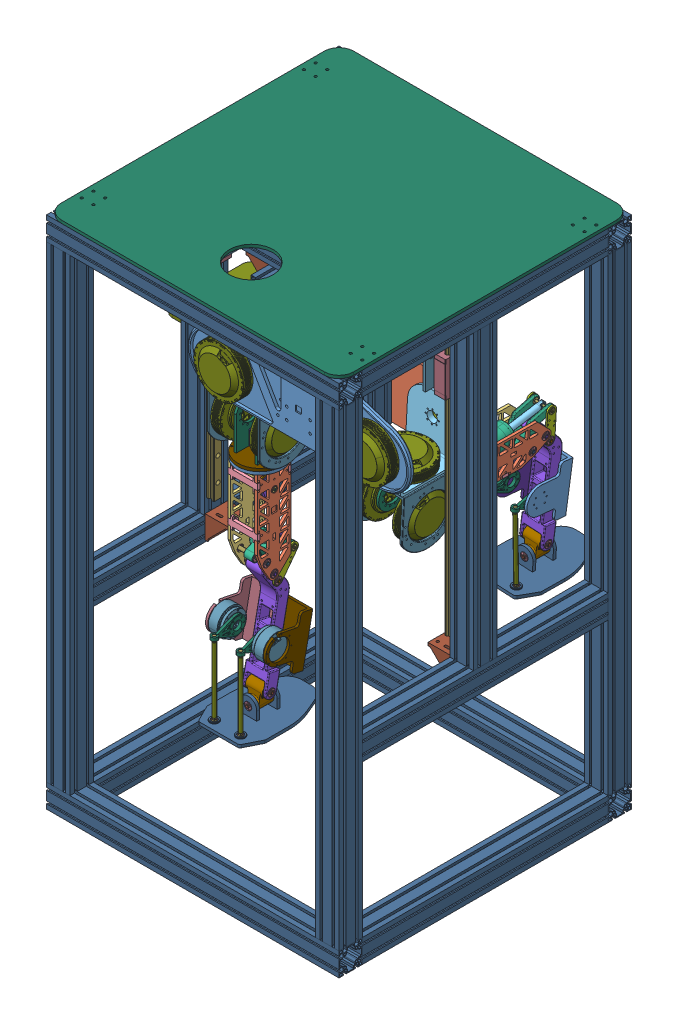
SolidWorks assembly 完整下肢, configuration 默认. Lengths in mm. (continued)
Mates (geometry in assembly coordinates): (continued)
- 重合58: coincident anti-aligned: plane of 腿髋转接架侧板V2-4 through (-333.8233 -333.6825 700.2525) normal (0 -1 0); plane of 腿髋转接架底座V2-2 through (-301.8233 -333.6825 652.2525) normal (0 1 0)
- 同心49: concentric aligned: cylinder of 腿髋转接架侧板V2-1 through (225.0525 -200.9494 601.8455) axis (-0.000625 -0.011709 -0.999931) radius 2.75; cylinder of 腿髋转接架底座V2-1 through (225.0318 -201.3358 568.8478) axis (-0.000625 -0.011709 -0.999931) radius 2.75
- 同心50: concentric aligned: cylinder of 腿髋转接架侧板V2-2 through (149.4212 -267.0042 602.6663) axis (-0.000625 -0.011709 -0.999931) radius 2.75; cylinder of 腿髋转接架底座V2-1 through (149.4006 -267.3906 569.6686) axis (-0.000625 -0.011709 -0.999931) radius 2.75
- 同心51: concentric aligned: cylinder of 腿髋转接架侧板V2-3 through (-265.8233 -283.6825 617.2525) axis (0 -1 0) radius 2.75; cylinder of 腿髋转接架底座V2-2 through (-265.8233 -316.6825 617.2525) axis (0 -1 0) radius 2.75
- 同心53: concentric aligned: cylinder of 腿髋转接架侧板V2-4 through (-337.8233 -283.6825 687.2525) axis (0 -1 0) radius 2.75; cylinder of 腿髋转接架底座V2-2 through (-337.8233 -316.6825 687.2525) axis (0 -1 0) radius 2.75
- 重合59: coincident anti-aligned: plane of 腿髋转接架侧板V2-3 through (-269.8233 -333.6825 604.2525) normal (0 -1 0); plane of 腿髋转接架底座V2-2 through (-301.8233 -333.6825 652.2525) normal (0 1 0)
- 重合61: coincident anti-aligned: plane of 腿髋转接架底座V2-2 through (-301.8233 -343.6825 652.2525) normal (0 -1 0); plane of 大腿主干_上板V2-1 through (-301.8233 -343.6825 652.2525) normal (0 1 0)
- 同心54: concentric anti-aligned: cylinder of 腿髋转接架底座V2-2 through (-301.8233 -343.6825 652.2525) axis (0 1 0) radius 75; cylinder of 大腿主干_上板V2-1 through (-301.8233 -343.6825 652.2525) axis (0 -1 0) radius 75
- 同心55: concentric aligned: cylinder of 腿髋转接架底座V2-2 through (-322.8233 -316.6825 652.2525) axis (0 -1 0) radius 2.75; cylinder of 大腿主干_上板V2-1 through (-322.8233 -343.6825 652.2525) axis (0 -1 0) radius 2.5
- 重合62: coincident anti-aligned: plane of 腿髋转接架底座V2-1 through (187.1993 -234.6794 542.26) normal (-0.000625 -0.011709 -0.999931); plane of 大腿主干_上板V2-2 through (187.1993 -234.6794 542.26) normal (0.000625 0.011709 0.999931)
- 同心56: concentric anti-aligned: cylinder of 腿髋转接架底座V2-1 through (187.1993 -234.6794 542.26) axis (0.000625 0.011709 0.999931) radius 75; cylinder of 大腿主干_上板V2-2 through (187.1993 -234.6794 542.26) axis (-0.000625 -0.011709 -0.999931) radius 75
- 同心57: concentric aligned: cylinder of 腿髋转接架底座V2-1 through (208.1863 -235.4834 569.2582) axis (-0.000625 -0.011709 -0.999931) radius 2.75; cylinder of 大腿主干_上板V2-2 through (208.1694 -235.7996 542.26) axis (-0.000625 -0.011709 -0.999931) radius 2.75
- 重合63: coincident anti-aligned: plane of 大腿主干_上板V2-2 through (187.1931 -234.7964 532.2607) normal (-0.000625 -0.011709 -0.999931); plane of 大腿主干_右侧板V2-1 through (-197.0913 -196.244 532.0497) normal (0.000625 0.011709 0.999931)
- 同心58: concentric anti-aligned: cylinder of 大腿主干_上板V2-2 through (233.968 -212.1438 541.9669) axis (-0.000625 -0.011709 -0.999931) radius 2.75; cylinder of 大腿主干_右侧板V2-1 through (233.948 -212.5184 509.9691) axis (0.000625 0.011709 0.999931) radius 2.5
- 同心59: concentric anti-aligned: cylinder of 大腿主干_上板V2-2 through (231.3011 -262.0691 542.5532) axis (-0.000625 -0.011709 -0.999931) radius 2.75; cylinder of 大腿主干_右侧板V2-1 through (231.281 -262.4438 510.5554) axis (0.000625 0.011709 0.999931) radius 2.5
- 重合64: coincident anti-aligned: plane of 大腿主干_上板V2-1 through (-301.8233 -353.6825 652.2525) normal (0 -1 0); plane of 大腿主干_右侧板V2-2 through (-687.617 -353.6825 634.2525) normal (0 1 0)
- 同心61: concentric anti-aligned: cylinder of 大腿主干_上板V2-1 through (-256.3233 -343.6825 627.2525) axis (0 -1 0) radius 2.75; cylinder of 大腿主干_右侧板V2-2 through (-256.3233 -375.6825 627.2525) axis (0 1 0) radius 2.5
- 同心62: concentric anti-aligned: line of 大腿主干_上板V2-1 through (-256.3233 -343.6825 677.2525) axis (0 -1 0); axis of 大腿主干_右侧板V2-2 through (-256.3233 -363.6825 677.2525) axis (0 1 0)
- 重合65: coincident anti-aligned: plane of 大腿主干_上板V2-2 through (187.1931 -234.7964 532.2607) normal (-0.000625 -0.011709 -0.999931); plane of 大腿主干_左侧板V2-1 through (-201.1451 -272.1306 532.9408) normal (0.000625 0.011709 0.999931)
- 同心63: concentric anti-aligned: cylinder of 大腿主干_上板V2-2 through (143.0976 -207.2896 541.9669) axis (-0.000625 -0.011709 -0.999931) radius 2.75; cylinder of 大腿主干_左侧板V2-1 through (143.0807 -207.6057 514.9688) axis (0.000625 0.011709 0.999931) radius 2.5
- 同心64: concentric anti-aligned: cylinder of 大腿主干_上板V2-2 through (140.4306 -257.2149 542.5532) axis (-0.000625 -0.011709 -0.999931) radius 2.75; cylinder of 大腿主干_左侧板V2-1 through (140.4137 -257.5311 515.555) axis (0.000625 0.011709 0.999931) radius 2.5
- 重合66: coincident anti-aligned: plane of 大腿主干_上板V2-1 through (-301.8233 -353.6825 652.2525) normal (0 -1 0); plane of 大腿主干_左侧板V2-2 through (-687.617 -353.6825 710.2525) normal (0 1 0)
- 同心65: concentric anti-aligned: cylinder of 大腿主干_上板V2-1 through (-347.3233 -343.6825 627.2525) axis (0 -1 0) radius 2.75; cylinder of 大腿主干_左侧板V2-2 through (-347.3233 -370.6825 627.2525) axis (0 1 0) radius 2.5
- 同心66: concentric anti-aligned: cylinder of 大腿主干_上板V2-1 through (-347.3233 -343.6825 677.2525) axis (0 -1 0) radius 2.75; circle of 大腿主干_左侧板V2-2
- 重合67: coincident anti-aligned: plane of 大腿主干_左侧板V2-1 through (109.5394 -282.471 212.8456) normal (-0.053339 -0.998508 0.011726); plane of 大腿侧板连接V2-4 through (134.6758 -280.5846 487.8267) normal (0.053339 0.998508 -0.011726)
- 重合68: coincident anti-aligned: plane of 大腿主干_左侧板V2-1 through (112.2717 -231.3226 487.2638) normal (0.000625 0.011709 0.999931); plane of 大腿侧板连接V2-4 through (134.1424 -290.5696 487.9439) normal (-0.000625 -0.011709 -0.999931)
- 重合69: coincident anti-aligned: plane of 大腿主干_左侧板V2-1 through (143.1703 -290.2887 552.9394) normal (0.998576 -0.053343 0); plane of 大腿侧板连接V2-4 through (143.1296 -291.0497 487.9439) normal (-0.998576 0.053343 0)
- 重合70: coincident anti-aligned: plane of 大腿主干_左侧板V2-1 through (109.5394 -282.471 212.8456) normal (-0.053339 -0.998508 0.011726); plane of 大腿侧板连接V2-1 through (134.5818 -282.3444 337.5398) normal (0.053339 0.998508 -0.011726)
- 重合71: coincident anti-aligned: plane of 大腿主干_左侧板V2-1 through (112.1777 -233.0825 336.977) normal (0.000625 0.011709 0.999931); plane of 大腿侧板连接V2-1 through (134.0484 -292.3295 337.6571) normal (-0.000625 -0.011709 -0.999931)
- 重合72: coincident anti-aligned: plane of 大腿主干_左侧板V2-1 through (143.1703 -290.2887 552.9394) normal (0.998576 -0.053343 0); plane of 大腿侧板连接V2-1 through (143.0356 -292.8096 337.6571) normal (-0.998576 0.053343 0)
- 重合74: coincident anti-aligned: plane of 大腿主干_左侧板V2-1 through (114.8445 -183.1601 506.6996) normal (0.053339 0.998508 -0.011726); plane of 大腿侧板连接V2-5 through (139.8089 -184.4937 506.6996) normal (-0.053339 -0.998508 0.011726)
- 重合75: coincident anti-aligned: plane of 大腿主干_左侧板V2-1 through (115.3654 -173.4092 486.5837) normal (0.000625 0.011709 0.999931); plane of 大腿侧板连接V2-5 through (140.3298 -174.7428 486.5837) normal (-0.000625 -0.011709 -0.999931)
- 重合76: coincident anti-aligned: plane of 大腿主干_左侧板V2-1 through (143.1703 -290.2887 552.9394) normal (0.998576 -0.053343 0); plane of 大腿侧板连接V2-5 through (149.3295 -174.9887 506.5824) normal (-0.998576 0.053343 0)
- 重合77: coincident anti-aligned: plane of 大腿主干_左侧板V2-2 through (-376.8233 -378.6825 604.2525) normal (0 0 -1); plane of 大腿侧板连接V2-2 through (-251.8233 -398.6825 604.2525) normal (0 0 1)
- 重合78: coincident anti-aligned: plane of 大腿主干_左侧板V2-2 through (-376.8233 -398.6825 594.2525) normal (0 1 0); plane of 大腿侧板连接V2-2 through (-251.8233 -398.6825 594.2525) normal (0 -1 0)
- 重合79: coincident anti-aligned: plane of 大腿主干_左侧板V2-2 through (-342.8233 -333.6825 710.2525) normal (1 0 0); plane of 大腿侧板连接V2-2 through (-342.8233 -398.6825 594.2525) normal (-1 0 0)
- 重合80: coincident anti-aligned: plane of 大腿主干_左侧板V2-2 through (-376.8233 -673.6825 700.2525) normal (0 0 1); plane of 大腿侧板连接V2-6 through (-351.8233 -398.6825 700.2525) normal (0 0 -1)
- 重合81: coincident anti-aligned: plane of 大腿主干_左侧板V2-2 through (-376.8233 -398.6825 652.2525) normal (0 1 0); plane of 大腿侧板连接V2-6 through (-351.8233 -398.6825 710.2525) normal (0 -1 0)
- 重合82: coincident anti-aligned: plane of 大腿主干_左侧板V2-2 through (-342.8233 -333.6825 710.2525) normal (1 0 0); plane of 大腿侧板连接V2-6 through (-342.8233 -398.6825 710.2525) normal (-1 0 0)
- 重合83: coincident anti-aligned: plane of 大腿主干_左侧板V2-2 through (-376.8233 -673.6825 700.2525) normal (0 0 1); plane of 大腿侧板连接V2-3 through (-351.8233 -548.9797 700.2525) normal (0 0 -1)
- 重合84: coincident anti-aligned: plane of 大腿主干_左侧板V2-2 through (-376.8233 -548.9797 652.2525) normal (0 1 0); plane of 大腿侧板连接V2-3 through (-351.8233 -548.9797 710.2525) normal (0 -1 0)
- 重合85: coincident anti-aligned: plane of 大腿主干_左侧板V2-2 through (-342.8233 -333.6825 710.2525) normal (1 0 0); plane of 大腿侧板连接V2-3 through (-342.8233 -548.9797 710.2525) normal (-1 0 0)
- 重合86: coincident anti-aligned: plane of 大腿主干_上板V2-1 through (-301.8233 -353.6825 652.2525) normal (0 -1 0); plane of 大腿主干_连接块-3 through (-302.8233 -353.6825 647.2525) normal (0 1 0)
- 重合87: coincident anti-aligned: plane of 大腿主干_左侧板V2-2 through (-342.8233 -333.6825 710.2525) normal (1 0 0); plane of 大腿主干_连接块-3 through (-342.8233 -353.6825 647.2525) normal (-1 0 0)
- 重合88: coincident anti-aligned: plane of 大腿主干_上板V2-1 through (-301.8233 -353.6825 652.2525) normal (0 -1 0); plane of 大腿主干_连接块-4 through (-300.8233 -353.6825 657.2525) normal (0 1 0)
- 重合89: coincident anti-aligned: plane of 大腿主干_右侧板V2-2 through (-260.8233 -333.6825 710.2525) normal (-1 0 0); plane of 大腿主干_连接块-4 through (-260.8233 -353.6825 657.2525) normal (1 0 0)
- 重合90: coincident anti-aligned: plane of 大腿主干_上板V2-2 through (187.1931 -234.7964 532.2607) normal (-0.000625 -0.011709 -0.999931); plane of 大腿主干_连接块-1 through (187.9249 -239.8423 532.3194) normal (0.000625 0.011709 0.999931)
- 重合91: coincident anti-aligned: plane of 大腿主干_右侧板V2-1 through (225.0535 -294.6628 552.9394) normal (-0.998576 0.053343 0); plane of 大腿主干_连接块-1 through (227.868 -241.976 532.3194) normal (0.998576 -0.053343 0)
- 重合93: coincident anti-aligned: plane of 大腿主干_上板V2-2 through (187.1931 -234.7964 532.2607) normal (-0.000625 -0.011709 -0.999931); plane of 大腿主干_连接块-2 through (186.4612 -229.7506 532.2021) normal (0.000625 0.011709 0.999931)
- 重合94: coincident anti-aligned: plane of 大腿主干_左侧板V2-1 through (143.1703 -290.2887 552.9394) normal (0.998576 -0.053343 0); plane of 大腿主干_连接块-2 through (146.5181 -227.6169 532.2021) normal (-0.998576 0.053343 0)
- 同心67: concentric anti-aligned: cylinder of 大腿主干_连接块-2 through (166.2004 -234.0978 496.2632) axis (0.000625 0.011709 0.999931) radius 2.5; cylinder of 大腿主干_上板V2-2 through (166.2292 -233.5592 542.26) axis (-0.000625 -0.011709 -0.999931) radius 2.5
- 同心68: concentric anti-aligned: cylinder of 大腿主干_上板V2-2 through (208.1694 -235.7996 542.26) axis (-0.000625 -0.011709 -0.999931) radius 2.75; cylinder of 大腿主干_连接块-1 through (208.1406 -236.3382 496.2632) axis (0.000625 0.011709 0.999931) radius 2.5
- 同心69: concentric anti-aligned: cylinder of 大腿主干_上板V2-1 through (-280.8233 -343.6825 652.2525) axis (0 -1 0) radius 2.75; cylinder of 大腿主干_连接块-4 through (-280.8233 -389.6825 652.2525) axis (0 1 0) radius 2.5
- 同心70: concentric anti-aligned: cylinder of 大腿主干_上板V2-1 through (-322.8233 -343.6825 652.2525) axis (0 -1 0) radius 2.5; cylinder of 大腿主干_连接块-3 through (-322.8233 -389.6825 652.2525) axis (0 1 0) radius 2.5
- 同心71: concentric aligned: cylinder of 大腿主干_左侧板V2-2 through (-238.8233 -423.6825 652.2525) axis (-1 0 0) radius 9.5; cylinder of 轴承_NSK635-4 through (-351.4346 -423.6825 652.2525) axis (-1 0 0) radius 9.5
- 重合95: coincident anti-aligned: plane of 大腿主干_左侧板V2-2 through (-352.8233 -432.1825 652.2525) normal (1 0 0); plane of 轴承_NSK635-4 through (-352.8233 -414.2003 651.6711) normal (-1 0 0)
- 同心72: concentric aligned: cylinder of 大腿主干_右侧板V2-2 through (-238.8233 -423.6825 652.2525) axis (-1 0 0) radius 9.5; cylinder of 轴承_NSK635-2 through (-255.4346 -423.6825 652.2525) axis (-1 0 0) radius 9.5
- 重合96: coincident anti-aligned: plane of 大腿主干_右侧板V2-2 through (-250.8233 -432.1825 652.2525) normal (-1 0 0); plane of 轴承_NSK635-2 through (-250.8233 -415.6975 651.7629) normal (1 0 0)
- 同心73: concentric aligned: cylinder of 大腿主干_右侧板V2-1 through (250.0596 -238.9767 462.2655) axis (-0.998576 0.053343 0) radius 9.5; cylinder of 轴承_NSK635-1 through (233.4719 -238.0906 462.2655) axis (-0.998576 0.053343 0) radius 9.5
- 重合97: coincident anti-aligned: plane of 大腿主干_右侧板V2-1 through (238.0714 -238.4361 453.7661) normal (-0.998576 0.053343 0); plane of 轴承_NSK635-1 through (238.4707 -230.9596 465.3357) normal (0.998576 -0.053343 0)
- 同心74: concentric aligned: cylinder of 大腿主干_左侧板V2-1 through (250.0596 -238.9767 462.2655) axis (-0.998576 0.053343 0) radius 9.5; cylinder of 轴承_NSK635-3 through (137.6086 -232.9697 462.2655) axis (-0.998576 0.053343 0) radius 9.5
- 重合98: coincident anti-aligned: plane of 大腿主干_左侧板V2-1 through (136.2166 -232.9951 453.7661) normal (0.998576 -0.053343 0); plane of 轴承_NSK635-3 through (136.6898 -224.1355 465.9114) normal (-0.998576 0.053343 0)
- 同心75: concentric anti-aligned: cylinder of 轴承_NSK635-1 through (233.4719 -238.0906 462.2655) axis (-0.998576 0.053343 0) radius 2.5; cylinder of 大腿_电机轴-1 through (133.2262 -232.7356 462.2655) axis (0.998576 -0.053343 0) radius 2.5
- 距离3: distance = 3 mm aligned: plane of 大腿_电机轴-1 through (241.0724 -238.4966 462.2655) normal (0.998576 -0.053343 0); plane of 轴承_NSK635-1 through (238.1998 -236.0313 463.225) normal (0.998576 -0.053343 0)
- 同心76: concentric anti-aligned: cylinder of 轴承_NSK635-4 through (-351.4346 -423.6825 652.2525) axis (-1 0 0) radius 2.5; cylinder of 大腿_电机轴-2 through (-355.8233 -423.6825 652.2525) axis (1 0 0) radius 2.5
- 距离4: distance = 3 mm aligned: plane of 轴承_NSK635-4 through (-352.8233 -419.69 652.0077) normal (-1 0 0); plane of 大腿_电机轴-2 through (-355.8233 -423.6825 652.2525) normal (-1 0 0)
- 同心77: concentric anti-aligned: cylinder of 大腿_电机轴-2 through (-355.8233 -423.6825 652.2525) axis (1 0 0) radius 2.5; cylinder of 轴套-5 through (-256.8233 -423.6825 652.2525) axis (-1 0 0) radius 2.5
- 重合101: coincident anti-aligned: plane of 轴承_NSK635-2 through (-256.8233 -419.69 652.0077) normal (-1 0 0); plane of 轴套-5 through (-256.8233 -423.6825 652.2525) normal (1 0 0)
- 同心78: concentric anti-aligned: cylinder of 大腿_电机轴-2 through (-355.8233 -423.6825 652.2525) axis (1 0 0) radius 2.5; cylinder of 轴套-6 through (-306.3233 -423.6825 652.2525) axis (-1 0 0) radius 2.5
- 重合102: coincident anti-aligned: plane of 轴承_NSK635-4 through (-346.8233 -421.1872 652.0995) normal (1 0 0); plane of 轴套-6 through (-346.8233 -423.6825 652.2525) normal (-1 0 0)
- 同心79: concentric aligned: cylinder of 大腿_电机轴-1 through (133.2262 -232.7356 462.2655) axis (0.998576 -0.053343 0) radius 2.5; cylinder of 轴套-4 through (191.6429 -235.8561 462.2655) axis (0.998576 -0.053343 0) radius 2.5
- 重合103: coincident anti-aligned: plane of 轴承_NSK635-1 through (232.2822 -234.328 463.8006) normal (-0.998576 0.053343 0); plane of 轴套-4 through (232.0852 -238.0165 462.2655) normal (0.998576 -0.053343 0)
- 同心80: concentric aligned: cylinder of 大腿_电机轴-1 through (133.2262 -232.7356 462.2655) axis (0.998576 -0.053343 0) radius 2.5; cylinder of 轴套-3 through (142.2133 -233.2156 462.2655) axis (0.998576 -0.053343 0) radius 2.5
- 重合104: coincident anti-aligned: plane of 轴承_NSK635-3 through (142.3365 -230.9104 463.225) normal (0.998576 -0.053343 0); plane of 轴套-3 through (142.2133 -233.2156 462.2655) normal (-0.998576 0.053343 0)
- 同心81: concentric anti-aligned: cylinder of 大腿主干_右侧板V2-1 through (335.5213 -271.003 255.8742) axis (-0.998576 0.053343 0) radius 11; cylinder of 轴承_NSK6900NR-5 through (235.2272 -265.6454 255.8742) axis (0.998576 -0.053343 0) radius 11
- 重合105: coincident anti-aligned: plane of 大腿主干_右侧板V2-1 through (234.8664 -265.6261 255.8742) normal (0.998576 -0.053343 0); plane of 轴承_NSK6900NR-5 through (234.8664 -265.6261 255.8742) normal (-0.998576 0.053343 0)
- 同心82: concentric aligned: cylinder of 大腿主干_右侧板V2-1 through (137.0641 -235.8762 212.2827) axis (0.998576 -0.053343 0) radius 11; cylinder of 轴承_NSK6900NR-6 through (236.5336 -241.1897 212.2827) axis (0.998576 -0.053343 0) radius 11
- 重合106: coincident anti-aligned: plane of 大腿主干_右侧板V2-1 through (236.1728 -241.1704 212.2827) normal (0.998576 -0.053343 0); plane of 轴承_NSK6900NR-6 through (236.1728 -241.1704 212.2827) normal (-0.998576 0.053343 0)
- 同心83: concentric aligned: cylinder of 大腿主干_左侧板V2-1 through (335.5213 -271.003 255.8742) axis (-0.998576 0.053343 0) radius 11; cylinder of 轴承_NSK6900NR-8 through (136.1459 -260.3526 255.8742) axis (-0.998576 0.053343 0) radius 11
- 重合107: coincident anti-aligned: plane of 大腿主干_左侧板V2-1 through (136.5066 -260.3719 255.8742) normal (-0.998576 0.053343 0); plane of 轴承_NSK6900NR-8 through (136.5066 -260.3719 255.8742) normal (0.998576 -0.053343 0)
- 同心84: concentric anti-aligned: cylinder of 大腿主干_左侧板V2-1 through (137.0641 -235.8762 212.2827) axis (0.998576 -0.053343 0) radius 11; cylinder of 轴承_NSK6900NR-11 through (137.4522 -235.8969 212.2827) axis (-0.998576 0.053343 0) radius 11
- 重合108: coincident anti-aligned: plane of 大腿主干_左侧板V2-1 through (137.813 -235.9162 212.2827) normal (-0.998576 0.053343 0); plane of 轴承_NSK6900NR-11 through (137.813 -235.9162 212.2827) normal (0.998576 -0.053343 0)
- 同心85: concentric anti-aligned: cylinder of 大腿主干_右侧板V2-2 through (-151.7748 -630.3812 677.2525) axis (-1 0 0) radius 11; cylinder of 轴承_NSK6900NR-7 through (-252.212 -630.3812 677.2525) axis (1 0 0) radius 11
- 重合109: coincident anti-aligned: plane of 大腿主干_右侧板V2-2 through (-252.5733 -630.3812 677.2525) normal (1 0 0); plane of 轴承_NSK6900NR-7 through (-252.5733 -630.3812 677.2525) normal (-1 0 0)
- 同心86: concentric aligned: cylinder of 大腿主干_右侧板V2-2 through (-351.8233 -673.6825 652.2525) axis (1 0 0) radius 11; cylinder of 轴承_NSK6900NR-9 through (-252.212 -673.6825 652.2525) axis (1 0 0) radius 11
- 重合110: coincident anti-aligned: plane of 大腿主干_右侧板V2-2 through (-252.5733 -673.6825 652.2525) normal (1 0 0); plane of 轴承_NSK6900NR-9 through (-252.5733 -673.6825 652.2525) normal (-1 0 0)
- 同心87: concentric aligned: cylinder of 大腿主干_左侧板V2-2 through (-151.7748 -630.3812 677.2525) axis (-1 0 0) radius 11; cylinder of 轴承_NSK6900NR-10 through (-351.4346 -630.3812 677.2525) axis (-1 0 0) radius 11
- 重合111: coincident anti-aligned: plane of 大腿主干_左侧板V2-2 through (-351.0733 -630.3812 677.2525) normal (-1 0 0); plane of 轴承_NSK6900NR-10 through (-351.0733 -630.3812 677.2525) normal (1 0 0)
- 同心88: concentric anti-aligned: cylinder of 大腿主干_左侧板V2-2 through (-351.8233 -673.6825 652.2525) axis (1 0 0) radius 11; cylinder of 轴承_NSK6900NR-12 through (-351.4346 -673.6825 652.2525) axis (-1 0 0) radius 11
- 重合112: coincident anti-aligned: plane of 大腿主干_左侧板V2-2 through (-351.0733 -673.6825 652.2525) normal (-1 0 0); plane of 轴承_NSK6900NR-12 through (-351.0733 -673.6825 652.2525) normal (1 0 0)
- 同心92: concentric aligned: cylinder of 膝盖上连杆_107.5V2-1 through (150.7363 -261.132 255.8742) axis (0.998576 -0.053343 0) radius 11; cylinder of 轴承_NSK6900NR-18 through (199.2784 -263.7251 255.8742) axis (0.998576 -0.053343 0) radius 11
- 重合116: coincident anti-aligned: plane of 膝盖上连杆_107.5V2-1 through (198.9176 -263.7058 255.8742) normal (0.998576 -0.053343 0); plane of 轴承_NSK6900NR-18 through (198.9176 -263.7058 255.8742) normal (-0.998576 0.053343 0)
- 同心93: concentric anti-aligned: cylinder of 膝盖上连杆_107.5V2-1 through (150.7363 -261.132 255.8742) axis (0.998576 -0.053343 0) radius 11; cylinder of 轴承_NSK6900NR-17 through (172.0946 -262.2729 255.8742) axis (-0.998576 0.053343 0) radius 11
- 重合117: coincident anti-aligned: plane of 膝盖上连杆_107.5V2-1 through (172.4554 -262.2922 255.8742) normal (-0.998576 0.053343 0); plane of 轴承_NSK6900NR-17 through (172.4554 -262.2922 255.8742) normal (0.998576 -0.053343 0)
- 同心94: concentric anti-aligned: cylinder of 膝盖上连杆_107.5V2-2 through (-336.8233 -630.3812 677.2525) axis (1 0 0) radius 11; cylinder of 轴承_NSK6900NR-19 through (-315.4346 -630.3812 677.2525) axis (-1 0 0) radius 11
- 重合118: coincident anti-aligned: plane of 膝盖上连杆_107.5V2-2 through (-315.0733 -630.3812 677.2525) normal (-1 0 0); plane of 轴承_NSK6900NR-19 through (-315.0733 -630.3812 677.2525) normal (1 0 0)
- 同心95: concentric aligned: cylinder of 膝盖上连杆_107.5V2-2 through (-336.8233 -630.3812 677.2525) axis (1 0 0) radius 11; cylinder of 轴承_NSK6900NR-20 through (-288.212 -630.3812 677.2525) axis (1 0 0) radius 11
- 重合119: coincident anti-aligned: plane of 膝盖上连杆_107.5V2-2 through (-288.5733 -630.3812 677.2525) normal (1 0 0); plane of 轴承_NSK6900NR-20 through (-288.5733 -630.3812 677.2525) normal (-1 0 0)
- 同心96: concentric anti-aligned: cylinder of 轴承_NSK6900NR-7 through (-252.212 -630.3812 677.2525) axis (1 0 0) radius 5; cylinder of 上连杆大腿轴-1 through (-355.8233 -630.3812 677.2525) axis (-1 0 0) radius 5
- 距离5: distance = 3 mm aligned: plane of 上连杆大腿轴-1 through (-247.8233 -625.3906 676.9465) normal (1 0 0); plane of 轴承_NSK6900NR-7 through (-250.8233 -629.0453 670.8912) normal (1 0 0)
- 同心97: concentric anti-aligned: cylinder of 轴承_NSK6900NR-5 through (235.2272 -265.6454 255.8742) axis (0.998576 -0.053343 0) radius 5; cylinder of 上连杆大腿轴-2 through (131.7634 -260.1185 255.8742) axis (-0.998576 0.053343 0) radius 5
- 距离6: distance = 3 mm aligned: plane of 轴承_NSK6900NR-5 through (236.7866 -262.486 250.2382) normal (0.998576 -0.053343 0); plane of 上连杆大腿轴-2 through (239.8559 -261.2689 257.793) normal (0.998576 -0.053343 0)
- 同心98: concentric aligned: cylinder of 轴承_NSK6900NR-19 through (-315.4346 -630.3812 677.2525) axis (-1 0 0) radius 5; cylinder of 上连杆大腿轴-1 through (-355.8233 -630.3812 677.2525) axis (-1 0 0) radius 5
- 同心99: concentric aligned: cylinder of 轴承_NSK6900NR-17 through (172.0946 -262.2729 255.8742) axis (-0.998576 0.053343 0) radius 5; cylinder of 上连杆大腿轴-2 through (131.7634 -260.1185 255.8742) axis (-0.998576 0.053343 0) radius 5
- 同心100: concentric anti-aligned: cylinder of 上连杆大腿轴-2 through (131.7634 -260.1185 255.8742) axis (-0.998576 0.053343 0) radius 5; cylinder of 轴套-8 through (200.6652 -263.7991 255.8742) axis (0.998576 -0.053343 0) radius 5
- 重合122: coincident anti-aligned: plane of 轴承_NSK6900NR-18 through (200.5282 -266.3628 249.9027) normal (0.998576 -0.053343 0); plane of 轴套-8 through (200.6652 -263.7991 255.8742) normal (-0.998576 0.053343 0)
- 同心101: concentric anti-aligned: cylinder of 上连杆大腿轴-2 through (131.7634 -260.1185 255.8742) axis (-0.998576 0.053343 0) radius 5; cylinder of 轴套-7 through (140.7506 -260.5986 255.8742) axis (0.998576 -0.053343 0) radius 5
- 重合123: coincident anti-aligned: plane of 轴承_NSK6900NR-17 through (170.7124 -262.1148 262.3736) normal (-0.998576 0.053343 0); plane of 轴套-7 through (170.7079 -262.1989 255.8742) normal (0.998576 -0.053343 0)
- 同心102: concentric aligned: cylinder of 上连杆大腿轴-1 through (-355.8233 -630.3812 677.2525) axis (-1 0 0) radius 5; cylinder of 轴套-10 through (-316.8233 -630.3812 677.2525) axis (-1 0 0) radius 5
- 重合124: coincident anti-aligned: plane of 轴承_NSK6900NR-19 through (-316.8233 -636.8163 676.336) normal (-1 0 0); plane of 轴套-10 through (-316.8233 -630.3812 677.2525) normal (1 0 0)
- 同心103: concentric aligned: cylinder of 上连杆大腿轴-1 through (-355.8233 -630.3812 677.2525) axis (-1 0 0) radius 5; cylinder of 轴套-9 through (-256.8233 -630.3812 677.2525) axis (-1 0 0) radius 5
- 重合125: coincident anti-aligned: plane of 轴承_NSK6900NR-20 through (-286.8233 -624.0859 675.6342) normal (1 0 0); plane of 轴套-9 through (-286.8233 -630.3812 677.2525) normal (-1 0 0)
- 重合126: coincident anti-aligned: plane of 轴承_NSK6900NR-10 through (-346.8233 -625.3906 676.9465) normal (1 0 0); plane of 轴套-10 through (-346.8233 -630.3812 677.2525) normal (-1 0 0)
- 重合127: coincident anti-aligned: plane of 轴承_NSK6900NR-5 through (230.7553 -262.9121 251.5388) normal (-0.998576 0.053343 0); plane of 轴套-8 through (230.6224 -265.3994 255.8742) normal (0.998576 -0.053343 0)
- 同心104: concentric anti-aligned: cylinder of 膝盖上连杆_107.5V2-2 through (-336.8233 -643.2766 570.5287) axis (1 0 0) radius 9.5; cylinder of 轴承_NSK635-6 through (-280.4346 -643.2766 570.5287) axis (-1 0 0) radius 9.5
- 同心105: concentric anti-aligned: cylinder of 膝盖上连杆_107.5V2-2 through (-336.8233 -643.2766 570.5287) axis (1 0 0) radius 9.5; cylinder of 轴承_NSK635-8 through (-326.4346 -643.2766 570.5287) axis (-1 0 0) radius 9.5
- 重合129: coincident aligned: plane of 膝盖上连杆_107.5V2-2 through (-321.8233 -611.2934 521.5177) normal (1 0 0); plane of 轴承_NSK635-8 through (-321.8233 -635.2916 570.0391) normal (1 0 0)
- 同心106: concentric anti-aligned: cylinder of 膝盖上连杆_107.5V2-1 through (154.7915 -185.2187 179.8677) axis (0.998576 -0.053343 0) radius 9.5; cylinder of 轴承_NSK635-7 through (211.1 -188.2267 179.8677) axis (-0.998576 0.053343 0) radius 9.5
- 同心107: concentric anti-aligned: cylinder of 膝盖上连杆_107.5V2-1 through (154.7915 -185.2187 179.8677) axis (0.998576 -0.053343 0) radius 9.5; cylinder of 轴承_NSK635-9 through (165.1655 -185.7729 179.8677) axis (-0.998576 0.053343 0) radius 9.5
- 重合131: coincident aligned: plane of 膝盖上连杆_107.5V2-1 through (172.8802 -127.7991 174.79) normal (0.998576 -0.053343 0); plane of 轴承_NSK635-9 through (170.1643 -178.642 182.9379) normal (0.998576 -0.053343 0)
- 同心108: concentric anti-aligned: cylinder of 膝关节下连杆_90-1 through (153.793 -185.1654 179.8677) axis (0.998576 -0.053343 0) radius 9.5; cylinder of 轴承_NSK635-11 through (154.1811 -185.1861 179.8677) axis (-0.998576 0.053343 0) radius 9.5
- 重合132: coincident anti-aligned: plane of 膝关节下连杆_90-1 through (152.341 -193.5998 179.9125) normal (0.998576 -0.053343 0); plane of 轴承_NSK635-11 through (152.801 -184.9892 189.3669) normal (-0.998576 0.053343 0)
- 同心109: concentric anti-aligned: cylinder of 膝关节下连杆_90-1 through (153.793 -185.1654 179.8677) axis (0.998576 -0.053343 0) radius 9.5; cylinder of 轴承_NSK635-13 through (222.0843 -188.8134 179.8677) axis (-0.998576 0.053343 0) radius 9.5
- 重合133: coincident anti-aligned: plane of 膝关节下连杆_90-1 through (226.2356 -197.5472 179.9125) normal (-0.998576 0.053343 0); plane of 轴承_NSK635-13 through (226.6946 -188.956 187.867) normal (0.998576 -0.053343 0)
- 同心110: concentric anti-aligned: cylinder of 膝关节下连杆_90-2 through (-265.8233 -643.2766 570.5287) axis (-1 0 0) radius 9.5; cylinder of 轴承_NSK635-12 through (-334.212 -643.2766 570.5287) axis (1 0 0) radius 9.5
- 重合134: coincident anti-aligned: plane of 膝关节下连杆_90-2 through (-338.8233 -650.0774 575.6277) normal (1 0 0); plane of 轴承_NSK635-12 through (-338.8233 -642.5448 562.5623) normal (-1 0 0)
- 同心111: concentric anti-aligned: cylinder of 膝关节下连杆_90-2 through (-265.8233 -643.2766 570.5287) axis (-1 0 0) radius 9.5; cylinder of 轴承_NSK635-10 through (-266.212 -643.2766 570.5287) axis (1 0 0) radius 9.5
- 重合135: coincident anti-aligned: plane of 膝关节下连杆_90-2 through (-264.8233 -650.0774 575.6277) normal (-1 0 0); plane of 轴承_NSK635-10 through (-264.8233 -641.9629 561.12) normal (1 0 0)
- 同心112: concentric aligned: cylinder of 轴承_NSK635-6 through (-280.4346 -643.2766 570.5287) axis (-1 0 0) radius 2.5; cylinder of 上下连杆轴-2 through (-261.8233 -643.2766 570.5287) axis (-1 0 0) radius 2.5
- 同心113: concentric anti-aligned: cylinder of 轴承_NSK635-9 through (165.1655 -185.7729 179.8677) axis (-0.998576 0.053343 0) radius 2.5; cylinder of 上下连杆轴-1 through (149.7987 -184.952 179.8677) axis (0.998576 -0.053343 0) radius 2.5
- 距离7: distance = 3 mm aligned: plane of 轴承_NSK635-13 through (226.6908 -189.0271 182.3675) normal (0.998576 -0.053343 0); plane of 上下连杆轴-1 through (229.6848 -189.2194 179.8677) normal (0.998576 -0.053343 0)
- 同心115: concentric anti-aligned: cylinder of 轴承_NSK635-12 through (-334.212 -643.2766 570.5287) axis (1 0 0) radius 2.5; cylinder of 上下连杆轴-2 through (-261.8233 -643.2766 570.5287) axis (-1 0 0) radius 2.5
- 距离8: distance = 3 mm aligned: plane of 上下连杆轴-2 through (-341.8233 -643.2766 570.5287) normal (-1 0 0); plane of 轴承_NSK635-12 through (-338.8233 -643.0479 568.0392) normal (-1 0 0)
- 同心116: concentric aligned: cylinder of 上下连杆轴-2 through (-261.8233 -643.2766 570.5287) axis (-1 0 0) radius 2.5; cylinder of 轴套-11 through (-327.8233 -643.2766 570.5287) axis (-1 0 0) radius 2.5
- 重合138: coincident anti-aligned: plane of 轴承_NSK635-8 through (-327.8233 -639.2841 570.2839) normal (-1 0 0); plane of 轴套-11 through (-327.8233 -643.2766 570.5287) normal (1 0 0)
- 重合139: coincident anti-aligned: plane of 轴承_NSK635-12 through (-332.8233 -642.9107 566.5455) normal (1 0 0); plane of 轴套-11 through (-332.8233 -643.2766 570.5287) normal (-1 0 0)
- 同心117: concentric aligned: cylinder of 上下连杆轴-2 through (-261.8233 -643.2766 570.5287) axis (-1 0 0) radius 2.5; cylinder of 轴套-13 through (-270.8233 -643.2766 570.5287) axis (-1 0 0) radius 2.5
- 重合140: coincident anti-aligned: plane of 轴承_NSK635-10 through (-270.8233 -642.9309 568.0527) normal (-1 0 0); plane of 轴套-13 through (-270.8233 -643.2766 570.5287) normal (1 0 0)
- 同心119: concentric aligned: cylinder of 上下连杆轴-1 through (149.7987 -184.952 179.8677) axis (0.998576 -0.053343 0) radius 2.5; cylinder of 轴套-14 through (215.7047 -188.4726 179.8677) axis (0.998576 -0.053343 0) radius 2.5
- 重合141: coincident anti-aligned: plane of 轴承_NSK635-13 through (220.7003 -188.6876 183.8674) normal (-0.998576 0.053343 0); plane of 轴套-14 through (220.6976 -188.7394 179.8677) normal (0.998576 -0.053343 0)
- 重合142: coincident anti-aligned: plane of 轴承_NSK635-7 through (215.8278 -186.1674 180.8271) normal (0.998576 -0.053343 0); plane of 轴套-14 through (215.7047 -188.4726 179.8677) normal (-0.998576 0.053343 0)
- 重合143: coincident aligned: plane of 膝盖上连杆_107.5V2-2 through (-281.8233 -611.2934 521.5177) normal (-1 0 0); plane of 轴承_NSK635-6 through (-281.8233 -633.7944 569.9473) normal (-1 0 0)
- 重合144: coincident aligned: plane of 膝盖上连杆_107.5V2-1 through (212.8233 -129.9328 174.79) normal (-0.998576 0.053343 0); plane of 轴承_NSK635-7 through (210.1812 -179.3925 183.5135) normal (-0.998576 0.053343 0)
- 同心120: concentric aligned: cylinder of 上下连杆轴-1 through (149.7987 -184.952 179.8677) axis (0.998576 -0.053343 0) radius 2.5; cylinder of 轴套-12 through (158.7858 -185.4321 179.8677) axis (0.998576 -0.053343 0) radius 2.5
- 重合145: coincident anti-aligned: plane of 轴承_NSK635-11 through (158.7876 -185.3998 182.3675) normal (0.998576 -0.053343 0); plane of 轴套-12 through (158.7858 -185.4321 179.8677) normal (-0.998576 0.053343 0)
- 同心121: concentric aligned: cylinder of 上下连杆轴-1 through (149.7987 -184.952 179.8677) axis (0.998576 -0.053343 0) radius 2.5; cylinder of 轴套-15 through (194.2353 -187.3258 179.8677) axis (0.998576 -0.053343 0) radius 2.5
- 重合146: coincident anti-aligned: plane of 轴承_NSK635-7 through (209.9103 -184.4641 181.4028) normal (-0.998576 0.053343 0); plane of 轴套-15 through (209.7132 -188.1526 179.8677) normal (0.998576 -0.053343 0)
- 同心122: concentric aligned: cylinder of 上下连杆轴-1 through (149.7987 -184.952 179.8677) axis (0.998576 -0.053343 0) radius 2.5; cylinder of 轴套-16 through (169.7702 -186.0189 179.8677) axis (0.998576 -0.053343 0) radius 2.5
- 重合147: coincident anti-aligned: plane of 轴承_NSK635-9 through (169.8933 -183.7136 180.8271) normal (0.998576 -0.053343 0); plane of 轴套-16 through (169.7702 -186.0189 179.8677) normal (-0.998576 0.053343 0)
- 同心123: concentric aligned: cylinder of 上下连杆轴-2 through (-261.8233 -643.2766 570.5287) axis (-1 0 0) radius 2.5; cylinder of 轴套-18 through (-306.3233 -643.2766 570.5287) axis (-1 0 0) radius 2.5
- 重合148: coincident anti-aligned: plane of 轴承_NSK635-8 through (-321.8233 -640.7813 570.3757) normal (1 0 0); plane of 轴套-18 through (-321.8233 -643.2766 570.5287) normal (-1 0 0)
- 同心124: concentric aligned: cylinder of 上下连杆轴-2 through (-261.8233 -643.2766 570.5287) axis (-1 0 0) radius 2.5; cylinder of 轴套-17 through (-281.8233 -643.2766 570.5287) axis (-1 0 0) radius 2.5
- 重合149: coincident anti-aligned: plane of 轴承_NSK635-6 through (-281.8233 -639.2841 570.2839) normal (-1 0 0); plane of 轴套-17 through (-281.8233 -643.2766 570.5287) normal (1 0 0)
- 同心125: concentric aligned: cylinder of 膝关节下连杆_90-1 through (148.9922 -275.036 180.3417) axis (0.998576 -0.053343 0) radius 11; cylinder of 轴承_NSK6900NR-21 through (220.5015 -278.856 180.3417) axis (0.998576 -0.053343 0) radius 11
- 重合150: coincident anti-aligned: plane of 膝关节下连杆_90-1 through (220.1407 -278.8367 180.3417) normal (0.998576 -0.053343 0); plane of 轴承_NSK6900NR-21 through (220.1407 -278.8367 180.3417) normal (-0.998576 0.053343 0)
- 同心126: concentric anti-aligned: cylinder of 膝关节下连杆_90-1 through (148.9922 -275.036 180.3417) axis (0.998576 -0.053343 0) radius 11; cylinder of 轴承_NSK6900NR-22 through (149.3803 -275.0567 180.3417) axis (-0.998576 0.053343 0) radius 11
- 重合151: coincident anti-aligned: plane of 膝关节下连杆_90-1 through (149.7411 -275.076 180.3417) normal (-0.998576 0.053343 0); plane of 轴承_NSK6900NR-22 through (149.7411 -275.076 180.3417) normal (0.998576 -0.053343 0)
- 同心127: concentric aligned: cylinder of 膝关节下连杆_90-2 through (-265.8233 -715.285 624.5175) axis (-1 0 0) radius 11; cylinder of 轴承_NSK6900NR-23 through (-337.4346 -715.285 624.5175) axis (-1 0 0) radius 11
- 重合152: coincident anti-aligned: plane of 膝关节下连杆_90-2 through (-337.0733 -715.285 624.5175) normal (-1 0 0); plane of 轴承_NSK6900NR-23 through (-337.0733 -715.285 624.5175) normal (1 0 0)
- 同心128: concentric anti-aligned: cylinder of 膝关节下连杆_90-2 through (-265.8233 -715.285 624.5175) axis (-1 0 0) radius 11; cylinder of 轴承_NSK6900NR-24 through (-266.212 -715.285 624.5175) axis (1 0 0) radius 11
- 重合153: coincident anti-aligned: plane of 膝关节下连杆_90-2 through (-266.5733 -715.285 624.5175) normal (1 0 0); plane of 轴承_NSK6900NR-24 through (-266.5733 -715.285 624.5175) normal (-1 0 0)
- 同心130: concentric anti-aligned: cylinder of 轴承_NSK635-13 through (222.0843 -188.8134 179.8677) axis (-0.998576 0.053343 0) radius 2.5; cylinder of 上下连杆轴-1 through (149.7987 -184.952 179.8677) axis (0.998576 -0.053343 0) radius 2.5
- 同心131: concentric anti-aligned: cylinder of 轴承_NSK6900NR-6 through (236.5336 -241.1897 212.2827) axis (0.998576 -0.053343 0) radius 5; cylinder of 大腿小腿轴-1 through (133.0698 -235.6628 212.2827) axis (-0.998576 0.053343 0) radius 5
- 距离9: distance = 3 mm aligned: plane of 轴承_NSK6900NR-6 through (238.093 -238.0303 206.6467) normal (0.998576 -0.053343 0); plane of 大腿小腿轴-1 through (241.1666 -236.7327 213.9945) normal (0.998576 -0.053343 0)
- 同心132: concentric anti-aligned: cylinder of 轴承_NSK6900NR-9 through (-252.212 -673.6825 652.2525) axis (1 0 0) radius 5; cylinder of 大腿小腿轴-2 through (-355.8233 -673.6825 652.2525) axis (-1 0 0) radius 5
- 距离10: distance = 3 mm aligned: plane of 轴承_NSK6900NR-9 through (-250.8233 -672.3466 645.8912) normal (1 0 0); plane of 大腿小腿轴-2 through (-247.8233 -668.6914 651.9551) normal (1 0 0)
- 同心133: concentric anti-aligned: cylinder of 轴承_NSK6900NR-21 through (220.5015 -278.856 180.3417) axis (0.998576 -0.053343 0) radius 5; cylinder of 下连杆小腿轴-1 through (144.9979 -274.8226 180.3417) axis (-0.998576 0.053343 0) radius 5
- 距离11: distance = 3 mm aligned: plane of 轴承_NSK6900NR-21 through (222.061 -275.6965 174.7057) normal (0.998576 -0.053343 0); plane of 下连杆小腿轴-1 through (225.1307 -274.4714 182.241) normal (0.998576 -0.053343 0)
- 同心134: concentric aligned: cylinder of 轴承_NSK6900NR-23 through (-337.4346 -715.285 624.5175) axis (-1 0 0) radius 5; cylinder of 下连杆小腿轴-2 through (-341.8233 -715.285 624.5175) axis (-1 0 0) radius 5
- 距离12: distance = 3 mm aligned: plane of 轴承_NSK6900NR-24 through (-264.8233 -713.9491 618.1562) normal (1 0 0); plane of 下连杆小腿轴-2 through (-261.8233 -710.2939 624.2201) normal (1 0 0)
- 同心135: concentric anti-aligned: cylinder of 小腿主干-1 through (157.0356 -236.943 212.2827) axis (0.998576 -0.053343 0) radius 11; cylinder of 轴承_NSK6900NR-25 through (158.4223 -237.0171 212.2827) axis (-0.998576 0.053343 0) radius 11
- 同心136: concentric anti-aligned: cylinder of 小腿主干-1 through (254.8413 -280.6903 180.3417) axis (-0.998576 0.053343 0) radius 11; cylinder of 轴承_NSK6900NR-28 through (213.5115 -278.4826 180.3417) axis (0.998576 -0.053343 0) radius 11
- 重合158: coincident anti-aligned: plane of 小腿主干-1 through (213.1507 -278.4633 180.3417) normal (0.998576 -0.053343 0); plane of 轴承_NSK6900NR-28 through (213.1507 -278.4633 180.3417) normal (-0.998576 0.053343 0)
- 重合159: coincident anti-aligned: plane of 小腿主干-1 through (158.7831 -237.0364 212.2827) normal (-0.998576 0.053343 0); plane of 轴承_NSK6900NR-25 through (158.7831 -237.0364 212.2827) normal (0.998576 -0.053343 0)
- 同心137: concentric aligned: cylinder of 轴承_NSK6900NR-27 through (156.3704 -275.4301 180.3417) axis (-0.998576 0.053343 0) radius 11; cylinder of 小腿主干-1 through (254.8413 -280.6903 180.3417) axis (-0.998576 0.053343 0) radius 11
- 同心138: concentric aligned: cylinder of 小腿主干-1 through (157.0356 -236.943 212.2827) axis (0.998576 -0.053343 0) radius 11; cylinder of 轴承_NSK6900NR-26 through (215.5635 -240.0695 212.2827) axis (0.998576 -0.053343 0) radius 11
- 重合161: coincident anti-aligned: plane of 小腿主干-1 through (215.2027 -240.0503 212.2827) normal (0.998576 -0.053343 0); plane of 轴承_NSK6900NR-26 through (215.2027 -240.0503 212.2827) normal (-0.998576 0.053343 0)
- 重合162: coincident anti-aligned: plane of 小腿主干-1 through (156.7311 -275.4494 180.3417) normal (-0.998576 0.053343 0); plane of 轴承_NSK6900NR-27 through (156.7311 -275.4494 180.3417) normal (0.998576 -0.053343 0)
- 同心139: concentric anti-aligned: cylinder of 大腿小腿轴-1 through (133.0698 -235.6628 212.2827) axis (-0.998576 0.053343 0) radius 5; cylinder of 轴承_NSK6900NR-26 through (215.5635 -240.0695 212.2827) axis (0.998576 -0.053343 0) radius 5
- 同心140: concentric anti-aligned: cylinder of 下连杆小腿轴-1 through (144.9979 -274.8226 180.3417) axis (-0.998576 0.053343 0) radius 5; cylinder of 轴承_NSK6900NR-28 through (213.5115 -278.4826 180.3417) axis (0.998576 -0.053343 0) radius 5
- 同心141: concentric anti-aligned: cylinder of 小腿主干-2 through (-331.8233 -673.6825 652.2525) axis (1 0 0) radius 11; cylinder of 轴承_NSK6900NR-29 through (-330.4346 -673.6825 652.2525) axis (-1 0 0) radius 11
- 重合163: coincident anti-aligned: plane of 小腿主干-2 through (-330.0733 -673.6825 652.2525) normal (-1 0 0); plane of 轴承_NSK6900NR-29 through (-330.0733 -673.6825 652.2525) normal (1 0 0)
- 同心142: concentric aligned: cylinder of 小腿主干-2 through (-331.8233 -673.6825 652.2525) axis (1 0 0) radius 11; cylinder of 轴承_NSK6900NR-32 through (-273.212 -673.6825 652.2525) axis (1 0 0) radius 11
- 重合164: coincident anti-aligned: plane of 小腿主干-2 through (-273.5733 -673.6825 652.2525) normal (1 0 0); plane of 轴承_NSK6900NR-32 through (-273.5733 -673.6825 652.2525) normal (-1 0 0)
- 同心143: concentric anti-aligned: cylinder of 小腿主干-2 through (-231.8233 -715.285 624.5175) axis (-1 0 0) radius 11; cylinder of 轴承_NSK6900NR-30 through (-273.212 -715.285 624.5175) axis (1 0 0) radius 11
- 重合165: coincident anti-aligned: plane of 小腿主干-2 through (-273.5733 -715.285 624.5175) normal (1 0 0); plane of 轴承_NSK6900NR-30 through (-273.5733 -715.285 624.5175) normal (-1 0 0)
- 同心144: concentric aligned: cylinder of 小腿主干-2 through (-231.8233 -715.285 624.5175) axis (-1 0 0) radius 11; cylinder of 轴承_NSK6900NR-31 through (-330.4346 -715.285 624.5175) axis (-1 0 0) radius 11
- 重合166: coincident anti-aligned: plane of 小腿主干-2 through (-330.0733 -715.285 624.5175) normal (-1 0 0); plane of 轴承_NSK6900NR-31 through (-330.0733 -715.285 624.5175) normal (1 0 0)
- 同心145: concentric anti-aligned: cylinder of 大腿小腿轴-2 through (-355.8233 -673.6825 652.2525) axis (-1 0 0) radius 5; cylinder of 轴承_NSK6900NR-32 through (-273.212 -673.6825 652.2525) axis (1 0 0) radius 5
- 同心146: concentric aligned: cylinder of 下连杆小腿轴-2 through (-341.8233 -715.285 624.5175) axis (-1 0 0) radius 5; cylinder of 轴承_NSK6900NR-31 through (-330.4346 -715.285 624.5175) axis (-1 0 0) radius 5
- 同心147: concentric anti-aligned: cylinder of 轴套-19 through (216.9502 -240.1436 212.2827) axis (0.998576 -0.053343 0) radius 5; cylinder of 大腿小腿轴-1 through (133.0698 -235.6628 212.2827) axis (-0.998576 0.053343 0) radius 5
- 同心148: concentric anti-aligned: cylinder of 大腿小腿轴-1 through (133.0698 -235.6628 212.2827) axis (-0.998576 0.053343 0) radius 5; cylinder of 轴套-21 through (142.057 -236.1429 212.2827) axis (0.998576 -0.053343 0) radius 5
- 同心149: concentric aligned: cylinder of 大腿小腿轴-2 through (-355.8233 -673.6825 652.2525) axis (-1 0 0) radius 5; cylinder of 轴套-20 through (-331.8233 -673.6825 652.2525) axis (-1 0 0) radius 5
- 同心150: concentric aligned: cylinder of 大腿小腿轴-2 through (-355.8233 -673.6825 652.2525) axis (-1 0 0) radius 5; cylinder of 轴套-22 through (-256.8233 -673.6825 652.2525) axis (-1 0 0) radius 5
- 重合168: coincident anti-aligned: plane of 轴承_NSK6900NR-32 through (-271.8233 -667.3455 650.8059) normal (1 0 0); plane of 轴套-22 through (-271.8233 -673.6825 652.2525) normal (-1 0 0)
- 重合169: coincident anti-aligned: plane of 轴承_NSK6900NR-29 through (-331.8233 -680.0903 651.1614) normal (-1 0 0); plane of 轴套-20 through (-331.8233 -673.6825 652.2525) normal (1 0 0)
- 重合170: coincident anti-aligned: plane of 轴承_NSK6900NR-12 through (-346.8233 -668.6919 651.9465) normal (1 0 0); plane of 轴套-20 through (-346.8233 -673.6825 652.2525) normal (-1 0 0)
- 重合171: coincident anti-aligned: plane of 轴承_NSK6900NR-25 through (157.0328 -236.9956 218.7825) normal (-0.998576 0.053343 0); plane of 轴套-21 through (157.0356 -236.943 212.2827) normal (0.998576 -0.053343 0)
- 重合172: coincident anti-aligned: plane of 轴承_NSK6900NR-26 through (216.8072 -242.8211 206.3615) normal (0.998576 -0.053343 0); plane of 轴套-19 through (216.9502 -240.1436 212.2827) normal (-0.998576 0.053343 0)
- 重合173: coincident anti-aligned: plane of 轴承_NSK6900NR-11 through (142.3033 -231.5323 214.2016) normal (0.998576 -0.053343 0); plane of 轴套-21 through (142.057 -236.1429 212.2827) normal (-0.998576 0.053343 0)
- 同心152: concentric aligned: cylinder of 下连杆小腿轴-2 through (-341.8233 -715.285 624.5175) axis (-1 0 0) radius 5; cylinder of 轴套-25 through (-270.8233 -715.285 624.5175) axis (-1 0 0) radius 5
- 重合175: coincident anti-aligned: plane of 轴承_NSK6900NR-23 through (-332.8233 -710.2944 624.2115) normal (1 0 0); plane of 轴套-23 through (-332.8233 -715.285 624.5175) normal (-1 0 0)
- 同心153: concentric anti-aligned: cylinder of 下连杆小腿轴-2 through (-341.8233 -715.285 624.5175) axis (-1 0 0) radius 5; cylinder of 轴套-23 through (-332.8233 -715.285 624.5175) axis (1 0 0) radius 5
- 重合176: coincident anti-aligned: plane of 轴承_NSK6900NR-30 through (-271.8233 -721.6928 623.4264) normal (1 0 0); plane of 轴套-25 through (-271.8233 -715.285 624.5175) normal (-1 0 0)
- 重合177: coincident anti-aligned: plane of 轴承_NSK6900NR-27 through (154.9808 -275.4086 186.8415) normal (-0.998576 0.053343 0); plane of 轴套-24 through (154.9836 -275.3561 180.3417) normal (0.998576 -0.053343 0)
- 同心154: concentric aligned: cylinder of 下连杆小腿轴-1 through (144.9979 -274.8226 180.3417) axis (-0.998576 0.053343 0) radius 5; cylinder of 轴套-24 through (154.9836 -275.3561 180.3417) axis (-0.998576 0.053343 0) radius 5
- 重合178: coincident anti-aligned: plane of 轴承_NSK6900NR-28 through (214.8954 -278.6092 186.8415) normal (0.998576 -0.053343 0); plane of 轴套-26 through (214.8982 -278.5566 180.3417) normal (-0.998576 0.053343 0)
- 同心155: concentric anti-aligned: cylinder of 下连杆小腿轴-1 through (144.9979 -274.8226 180.3417) axis (-0.998576 0.053343 0) radius 5; cylinder of 轴套-26 through (214.8982 -278.5566 180.3417) axis (0.998576 -0.053343 0) radius 5
- 同心156: concentric anti-aligned: cylinder of 小腿主干-1 through (208.001 -595.1387 174.8875) axis (-0.998576 0.053343 0) radius 11; cylinder of 轴承_NSK6900NR-34 through (207.6129 -595.1179 174.8875) axis (0.998576 -0.053343 0) radius 11
- 重合179: coincident anti-aligned: plane of 小腿主干-1 through (207.2521 -595.0987 174.8875) normal (0.998576 -0.053343 0); plane of 轴承_NSK6900NR-34 through (207.2521 -595.0987 174.8875) normal (-0.998576 0.053343 0)
- 同心157: concentric anti-aligned: cylinder of 小腿主干-1 through (128.1149 -590.8713 174.8875) axis (0.998576 -0.053343 0) radius 11; cylinder of 轴承_NSK6900NR-36 through (128.5031 -590.892 174.8875) axis (-0.998576 0.053343 0) radius 11
- 重合180: coincident anti-aligned: plane of 小腿主干-1 through (128.8639 -590.9113 174.8875) normal (-0.998576 0.053343 0); plane of 轴承_NSK6900NR-36 through (128.8639 -590.9113 174.8875) normal (0.998576 -0.053343 0)
- 同心158: concentric anti-aligned: cylinder of 小腿主干-2 through (-261.8233 -1030.6139 652.2525) axis (-1 0 0) radius 11; cylinder of 轴承_NSK6900NR-35 through (-262.212 -1030.6139 652.2525) axis (1 0 0) radius 11
- 重合181: coincident anti-aligned: plane of 小腿主干-2 through (-262.5733 -1030.6139 652.2525) normal (1 0 0); plane of 轴承_NSK6900NR-35 through (-262.5733 -1030.6139 652.2525) normal (-1 0 0)
- 同心159: concentric anti-aligned: cylinder of 小腿主干-2 through (-341.8233 -1030.6139 652.2525) axis (1 0 0) radius 11; cylinder of 轴承_NSK6900NR-33 through (-341.4346 -1030.6139 652.2525) axis (-1 0 0) radius 11
- 重合182: coincident anti-aligned: plane of 小腿主干-2 through (-341.0733 -1030.6139 652.2525) normal (-1 0 0); plane of 轴承_NSK6900NR-33 through (-341.0733 -1030.6139 652.2525) normal (1 0 0)
- 同心160: concentric anti-aligned: cylinder of 脚踝十字连接-1 through (-272.8233 -1030.6139 652.2525) axis (-1 0 0) radius 11; cylinder of 轴承_NSK6900NR-38 through (-274.212 -1030.6139 652.2525) axis (1 0 0) radius 11
- 重合183: coincident anti-aligned: plane of 脚踝十字连接-1 through (-274.5733 -1030.6139 652.2525) normal (1 0 0); plane of 轴承_NSK6900NR-38 through (-274.5733 -1030.6139 652.2525) normal (-1 0 0)
- 同心161: concentric aligned: cylinder of 脚踝十字连接-1 through (-272.8233 -1030.6139 652.2525) axis (-1 0 0) radius 11; cylinder of 轴承_NSK6900NR-37 through (-329.4346 -1030.6139 652.2525) axis (-1 0 0) radius 11
- 重合184: coincident anti-aligned: plane of 脚踝十字连接-1 through (-329.0733 -1030.6139 652.2525) normal (-1 0 0); plane of 轴承_NSK6900NR-37 through (-329.0733 -1030.6139 652.2525) normal (1 0 0)
